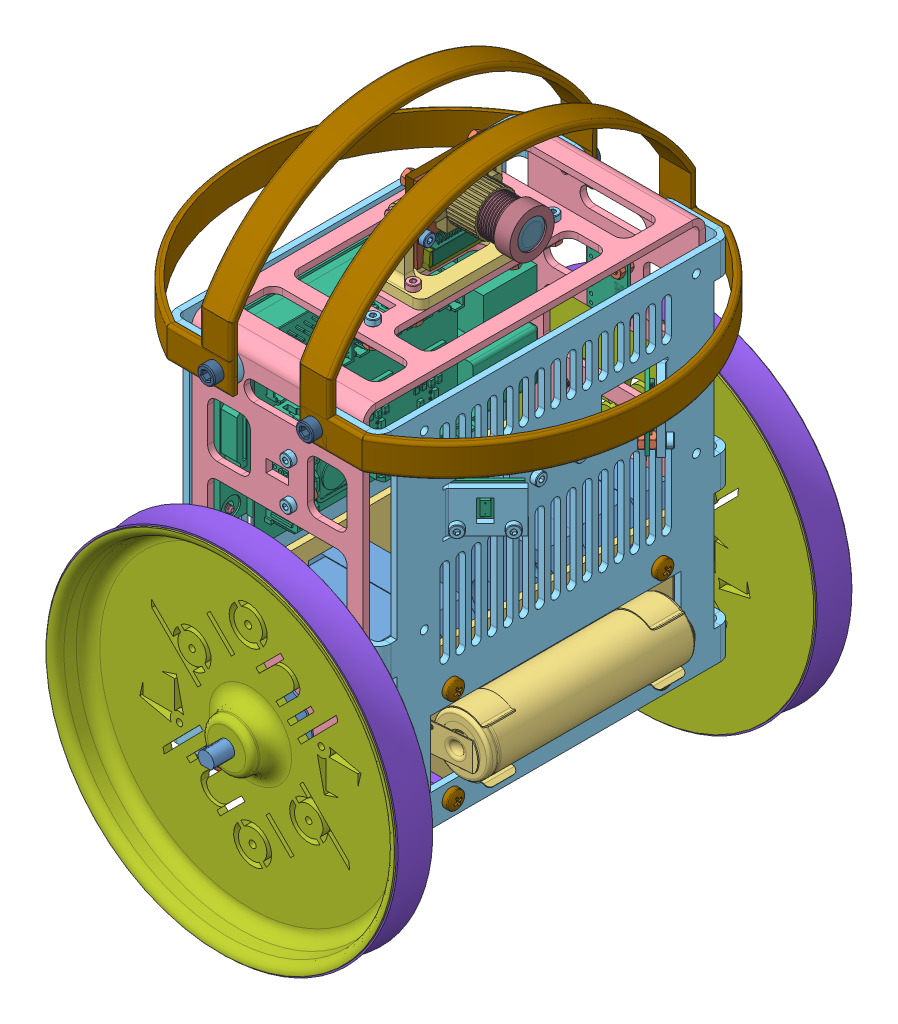
SolidWorks assembly irys4, configuration Domyślna. Lengths in mm. (continued)
Mates (geometry in assembly coordinates): (continued)
- Koncentryczne66: concentric aligned: cylinder of bumper-2 through (-57.7578 82.3211 -37.682) axis (0 0 1) radius 1.5; cylinder of bumper-4 through (-57.7578 82.3211 -37.75) axis (0 0 1) radius 1.5
- Wspólnie32: coincident: line of front-1 through (-57.7578 77.3211 -35.75) axis (-1 0 0); plane of bumper-4 through (-52.7604 77.3184 -35.75) normal (0 0 1)
- Koncentryczne67: concentric aligned: cylinder of bumper-3 through (-26.7578 82.3211 -37.75) axis (0 0 1) radius 1.5; cylinder of bumper-5 through (-26.7578 82.3211 -37.75) axis (0 0 1) radius 1.5
- Wspólnie33: coincident: line of front-2 through (-26.7578 87.3211 -35.75) axis (1 0 0); plane of bumper-5 through (-21.7734 77.3055 -35.75) normal (0 0 1)
- Wspólnie34: coincident anti-aligned: plane of topframe-1 through (-42.2578 90.6087 -127.75) normal (0 1 0); plane of camera_mounted-1/mount1-1 through (-40.7578 90.6087 2.1027) normal (0 -1 0)
- Koncentryczne70: concentric aligned: cylinder of front-2 through (0.677 52.3211 42.6028) axis (0.707107 0 0.707107) radius 1.25; cylinder of m2_x_0_4mm_thread_6mm_long_sock-2 through (3.5055 52.3211 45.4313) axis (0.707107 0 0.707107) radius 1.9
- Wspólnie35: coincident anti-aligned: plane of front-2 through (-34.9258 82.3211 81.0341) normal (0.707107 0 0.707107); plane of m2_x_0_4mm_thread_6mm_long_sock-2 through (2.0912 52.3211 44.017) normal (-0.707107 0 -0.707107)
- Koncentryczne71: concentric aligned: cylinder of front-2 through (-8.3032 52.3211 51.5831) axis (0.707107 0 0.707107) radius 1.25; cylinder of m2_x_0_4mm_thread_6mm_long_sock-1 through (-5.4748 52.3211 54.4115) axis (0.707107 0 0.707107) radius 1.9
- Wspólnie36: coincident anti-aligned: plane of front-2 through (-34.9258 82.3211 81.0341) normal (0.707107 0 0.707107); plane of m2_x_0_4mm_thread_6mm_long_sock-1 through (-6.889 52.3211 52.9973) normal (-0.707107 0 -0.707107)
- Koncentryczne76: concentric aligned: cylinder of front-1 through (-77.0454 33.0917 64.6663) axis (1 0 0) radius 1.25; cylinder of M2 x 0.4mm Thread 10mm LONG SOCKET HEAD CAP SCREW-1 through (-78.0454 33.0917 64.6663) axis (1 0 0) radius 1.9
- Wspólnie43: coincident anti-aligned: plane of front-1 through (-76.0454 82.3211 -50.75) normal (-1 0 0); plane of M2 x 0.4mm Thread 10mm LONG SOCKET HEAD CAP SCREW-1 through (-76.0454 33.0917 64.6663) normal (1 0 0)
- Koncentryczne77: concentric aligned: cylinder of front-1 through (-77.0454 82.1645 64.6663) axis (1 0 0) radius 1.25; cylinder of M2 x 0.4mm Thread 10mm LONG SOCKET HEAD CAP SCREW-2 through (-78.0454 82.1645 64.6663) axis (1 0 0) radius 1.9
- Wspólnie44: coincident anti-aligned: plane of front-1 through (-76.0454 82.3211 -50.75) normal (-1 0 0); plane of M2 x 0.4mm Thread 10mm LONG SOCKET HEAD CAP SCREW-2 through (-76.0454 82.1645 64.6663) normal (1 0 0)
- Koncentryczne82: concentric anti-aligned: cylinder of m2_x_0_4mm_thread_6mm_long_sock-2 through (3.5055 52.3211 45.4313) axis (0.707107 0 0.707107) radius 1.9; cylinder of ToF_nut-1/m2_x_0_4mm_thread_hex_nut-1 through (-2.307 52.3211 39.6188) axis (-0.707107 0 -0.707107) radius 0.7402
- Koncentryczne83: concentric anti-aligned: cylinder of m2_x_0_4mm_thread_6mm_long_sock-1 through (-5.4748 52.3211 54.4115) axis (0.707107 0 0.707107) radius 1.9; cylinder of ToF_nut-1/m2_x_0_4mm_thread_hex_nut-4 through (-9.4346 52.3211 50.4517) axis (-0.707107 0 -0.707107) radius 1
- Wspólnie49: coincident anti-aligned: plane of front-2 through (-36.34 82.3211 79.6199) normal (-0.707107 0 -0.707107); plane of ToF_nut-1/m2_x_0_4mm_thread_hex_nut-3 through (1.973 50.9159 41.3069) normal (0.707107 0 0.707107)
- Koncentryczne84: concentric aligned: cylinder of front-2 through (0.9091 52.3211 -2.1989) axis (0.707107 0 -0.707107) radius 1.25; cylinder of ToF_nut-2/m2_x_0_4mm_thread_hex_nut-2 through (-0.9436 52.3211 -0.3463) axis (0.707107 0 -0.707107) radius 0.7402
- Koncentryczne85: concentric aligned: cylinder of front-2 through (-8.0712 52.3211 -11.1792) axis (0.707107 0 -0.707107) radius 1.25; cylinder of ToF_nut-2/m2_x_0_4mm_thread_hex_nut-3 through (-8.0712 52.3211 -11.1792) axis (0.707107 0 -0.707107) radius 0.7402
- Wspólnie51: coincident anti-aligned: plane of front-2 through (64.3012 82.3211 61.1932) normal (-0.707107 0 0.707107); plane of ToF_nut-2/m2_x_0_4mm_thread_hex_nut-4 through (-0.3869 50.9159 -3.4949) normal (0.707107 0 -0.707107)
- Koncentryczne86: concentric aligned: cylinder of front-2 through (-10.4701 52.3211 26.6) axis (1 0 0) radius 1.25; cylinder of ToF_nut-3/m2_x_0_4mm_thread_hex_nut-4 through (-10.4701 52.3211 26.6) axis (1 0 0) radius 0.7402
- Koncentryczne87: concentric aligned: cylinder of front-2 through (-10.4701 52.3211 13.9) axis (1 0 0) radius 1.25; cylinder of ToF_nut-3/m2_x_0_4mm_thread_hex_nut-3 through (-10.4701 52.3211 13.9) axis (1 0 0) radius 0.7402
- Wspólnie52: coincident anti-aligned: plane of front-2 through (-10.4701 82.3211 91.25) normal (-1 0 0); plane of ToF_nut-3/m2_x_0_4mm_thread_hex_nut-3 through (-10.4701 50.9159 12.0673) normal (1 0 0)
- Koncentryczne92: concentric aligned: cylinder of front-2 through (-8.0712 52.3211 -11.1792) axis (0.707107 0 -0.707107) radius 1.25; cylinder of m2_x_0_4mm_thread_6mm_long_sock-4 through (-5.2428 52.3211 -14.0076) axis (0.707107 0 -0.707107) radius 1.9
- Koncentryczne93: concentric aligned: cylinder of front-2 through (0.9091 52.3211 -2.1989) axis (0.707107 0 -0.707107) radius 1.25; cylinder of m2_x_0_4mm_thread_6mm_long_sock-6 through (3.7375 52.3211 -5.0274) axis (0.707107 0 -0.707107) radius 1.9
- Koncentryczne94: concentric aligned: cylinder of front-2 through (-10.4701 52.3211 13.9) axis (1 0 0) radius 1.25; cylinder of m2_x_0_4mm_thread_6mm_long_sock-3 through (-6.4701 52.3211 13.9) axis (1 0 0) radius 1.9
- Koncentryczne95: concentric aligned: cylinder of front-2 through (-10.4701 52.3211 26.6) axis (1 0 0) radius 1.25; cylinder of m2_x_0_4mm_thread_6mm_long_sock-5 through (-6.4701 52.3211 26.6) axis (1 0 0) radius 1.9
- Wspólnie55: coincident anti-aligned: plane of front-2 through (-8.4701 82.3211 91.25) normal (1 0 0); plane of m2_x_0_4mm_thread_6mm_long_sock-5 through (-8.4701 52.3211 26.6) normal (-1 0 0)
- Wspólnie57: coincident anti-aligned: plane of front-2 through (65.7154 82.3211 59.779) normal (0.707107 0 -0.707107); plane of m2_x_0_4mm_thread_6mm_long_sock-4 through (-6.657 52.3211 -12.5934) normal (-0.707107 0 0.707107)
- Wspólnie58: coincident: plane of front-2 through (65.7154 82.3211 59.779) normal (0.707107 0 -0.707107); moEndPointRef_w of m2_x_0_4mm_thread_6mm_long_sock-6
- Wspólnie59: coincident anti-aligned: plane of front-2 through (-8.4701 82.3211 91.25) normal (1 0 0); plane of m2_x_0_4mm_thread_6mm_long_sock-3 through (-8.4701 52.3211 13.9) normal (-1 0 0)
- Koncentryczne96: concentric aligned: cylinder of topframe-1 through (-37.7578 90.6087 -8.1) axis (0 1 0) radius 1.25; cylinder of ToF_nut-4/m2_x_0_4mm_thread_hex_nut-3 through (-37.7578 88.6087 -8.1) axis (0 1 0) radius 0.7402
- Koncentryczne97: concentric aligned: cylinder of camera_mounted-1/mount1-1 through (-37.7578 90.6087 4.6) axis (0 1 0) radius 1.05; cylinder of ToF_nut-4/m2_x_0_4mm_thread_hex_nut-4 through (-37.7578 88.6087 4.6) axis (0 1 0) radius 0.7402
- Wspólnie60: coincident anti-aligned: plane of topframe-1 through (-42.2578 88.6087 -127.75) normal (0 -1 0); plane of ToF_nut-4/m2_x_0_4mm_thread_hex_nut-3 through (-36.3526 88.6087 -9.9327) normal (0 1 0)
- Koncentryczne98: concentric aligned: cylinder of topframe-1 through (-37.7578 90.6087 48.6) axis (0 1 0) radius 1.25; cylinder of ToF_nut-5/m2_x_0_4mm_thread_hex_nut-4 through (-37.7578 88.6087 48.6) axis (0 1 0) radius 0.7402
- Koncentryczne99: concentric aligned: cylinder of camera_mounted-1/mount1-1 through (-37.7578 90.6087 35.9) axis (0 1 0) radius 1.05; cylinder of ToF_nut-5/m2_x_0_4mm_thread_hex_nut-3 through (-37.7578 88.6087 35.9) axis (0 1 0) radius 0.7402
- Wspólnie61: coincident anti-aligned: plane of topframe-1 through (-42.2578 88.6087 -127.75) normal (0 -1 0); plane of ToF_nut-5/m2_x_0_4mm_thread_hex_nut-4 through (-36.3526 88.6087 46.7673) normal (0 1 0)
- Koncentryczne100: concentric anti-aligned: cylinder of camera_mounted-1/mount1-1 through (-37.7578 90.6087 35.9) axis (0 1 0) radius 1.05; cylinder of M2 x 0.4mm Thread 10mm LONG SOCKET HEAD CAP SCREW-4 through (-37.7578 95.6087 35.9) axis (0 -1 0) radius 1.9
- Koncentryczne102: concentric anti-aligned: cylinder of camera_mounted-1/mount1-1 through (-37.7578 90.6087 4.6) axis (0 1 0) radius 1.05; cylinder of M2 x 0.4mm Thread 10mm LONG SOCKET HEAD CAP SCREW-3 through (-37.7578 95.6087 4.6) axis (0 -1 0) radius 1.9
- Wspólnie62: coincident anti-aligned: plane of camera_mounted-1/mount1-1 through (-40.7578 93.6087 7.7527) normal (0 1 0); plane of M2 x 0.4mm Thread 10mm LONG SOCKET HEAD CAP SCREW-3 through (-37.7578 93.6087 4.6) normal (0 -1 0)
- Wspólnie64: coincident anti-aligned: plane of camera_mounted-1/mount1-1 through (-40.7578 93.6087 7.7527) normal (0 1 0); plane of M2 x 0.4mm Thread 10mm LONG SOCKET HEAD CAP SCREW-4 through (-37.7578 93.6087 35.9) normal (0 -1 0)
- Koncentryczne103: concentric aligned: cylinder of topframe-1 through (-37.7578 90.6087 -8.1) axis (0 1 0) radius 1.25; cylinder of m2_x_0_4mm_thread_6mm_long_sock-8 through (-37.7578 92.6087 -8.1) axis (0 1 0) radius 1.9
- Koncentryczne104: concentric aligned: cylinder of topframe-1 through (-37.7578 90.6087 48.6) axis (0 1 0) radius 1.25; cylinder of m2_x_0_4mm_thread_6mm_long_sock-7 through (-37.7578 92.6087 48.6) axis (0 1 0) radius 1.9
- Wspólnie65: coincident anti-aligned: plane of topframe-1 through (-42.2578 90.6087 -127.75) normal (0 1 0); plane of m2_x_0_4mm_thread_6mm_long_sock-7 through (-37.7578 90.6087 48.6) normal (0 -1 0)
- Wspólnie66: coincident anti-aligned: plane of topframe-1 through (-42.2578 90.6087 -127.75) normal (0 1 0); plane of m2_x_0_4mm_thread_6mm_long_sock-8 through (-37.7578 90.6087 -8.1) normal (0 -1 0)
- Koncentryczne105: concentric anti-aligned: cylinder of topframe-1 through (-37.7578 66.6711 74.25) axis (0 0 1) radius 1.25; cylinder of ToF_nut-6/m2_x_0_4mm_thread_hex_nut-3 through (-37.7578 66.6711 70.65) axis (0 0 -1) radius 1
- Koncentryczne106: concentric aligned: cylinder of topframe-1 through (-37.7578 53.9711 74.25) axis (0 0 1) radius 1.25; cylinder of ToF_nut-6/m2_x_0_4mm_thread_hex_nut-4 through (-37.7578 53.9711 72.25) axis (0 0 1) radius 0.7402
- Wspólnie67: coincident anti-aligned: plane of topframe-1 through (-42.2578 289.3211 72.25) normal (0 0 -1); plane of ToF_nut-6/m2_x_0_4mm_thread_hex_nut-4 through (-36.3526 55.8038 72.25) normal (0 0 1)
- Koncentryczne107: concentric anti-aligned: cylinder of topframe-1 through (-37.7578 53.9711 -33.75) axis (0 0 -1) radius 1.25; cylinder of ToF_nut-7/vl53l1x-1 through (-37.7578 53.9711 -30.15) axis (0 0 1) radius 1.0922
- Koncentryczne108: concentric aligned: cylinder of topframe-1 through (-37.7578 66.6711 -33.75) axis (0 0 -1) radius 1.25; cylinder of ToF_nut-7/m2_x_0_4mm_thread_hex_nut-4 through (-37.7578 66.6711 -31.75) axis (0 0 -1) radius 0.7402
- Wspólnie68: coincident anti-aligned: plane of topframe-1 through (-42.2578 -6.6789 -31.75) normal (0 0 1); plane of ToF_nut-7/m2_x_0_4mm_thread_hex_nut-3 through (-36.3526 52.1384 -31.75) normal (0 0 -1)
- Koncentryczne109: concentric aligned: cylinder of front-1 through (-76.2123 52.3211 -11.0831) axis (-0.707107 0 -0.707107) radius 1.25; cylinder of ToF_nut-8/m2_x_0_4mm_thread_hex_nut-4 through (-76.2123 52.3211 -11.0831) axis (-0.707107 0 -0.707107) radius 0.7402
- Koncentryczne110: concentric anti-aligned: cylinder of front-1 through (-85.1925 52.3211 -2.1028) axis (-0.707107 0 -0.707107) radius 1.25; cylinder of ToF_nut-8/m2_x_0_4mm_thread_hex_nut-3 through (-84.0612 52.3211 -0.9715) axis (0.707107 0 0.707107) radius 1
- Wspólnie69: coincident anti-aligned: plane of front-1 through (-48.1755 82.3211 -39.1199) normal (0.707107 0 0.707107); plane of ToF_nut-8/m2_x_0_4mm_thread_hex_nut-3 through (-86.4885 50.9159 -0.8069) normal (-0.707107 0 -0.707107)
- Koncentryczne111: concentric aligned: cylinder of front-1 through (-74.0454 52.3211 13.9) axis (-1 0 0) radius 1.25; cylinder of ToF_nut-9/m2_x_0_4mm_thread_hex_nut-4 through (-74.0454 52.3211 13.9) axis (-1 0 0) radius 0.7402
- Koncentryczne112: concentric aligned: cylinder of front-1 through (-74.0454 52.3211 26.6) axis (-1 0 0) radius 1.25; cylinder of ToF_nut-9/m2_x_0_4mm_thread_hex_nut-3 through (-74.0454 52.3211 26.6) axis (-1 0 0) radius 0.7402
- Wspólnie70: coincident anti-aligned: plane of front-1 through (-74.0454 82.3211 -50.75) normal (1 0 0); plane of ToF_nut-9/m2_x_0_4mm_thread_hex_nut-4 through (-74.0454 50.9159 15.7327) normal (-1 0 0)
- Koncentryczne113: concentric aligned: cylinder of front-1 through (-76.4443 52.3211 51.6792) axis (-0.707107 0 0.707107) radius 1.25; cylinder of ToF_nut-10/m2_x_0_4mm_thread_hex_nut-3 through (-76.4443 52.3211 51.6792) axis (-0.707107 0 0.707107) radius 0.7402
- Koncentryczne114: concentric aligned: cylinder of front-1 through (-85.4246 52.3211 42.6989) axis (-0.707107 0 0.707107) radius 1.25; cylinder of ToF_nut-10/m2_x_0_4mm_thread_hex_nut-4 through (-85.4246 52.3211 42.6989) axis (-0.707107 0 0.707107) radius 0.7402
- Wspólnie71: coincident anti-aligned: plane of front-1 through (-148.8167 82.3211 -20.6932) normal (0.707107 0 -0.707107); plane of ToF_nut-10/m2_x_0_4mm_thread_hex_nut-4 through (-84.1286 50.9159 43.9949) normal (-0.707107 0 0.707107)
- Koncentryczne115: concentric aligned: cylinder of front-1 through (-76.2123 52.3211 -11.0831) axis (-0.707107 0 -0.707107) radius 1.25; cylinder of m2_x_0_4mm_thread_6mm_long_sock-9 through (-79.0407 52.3211 -13.9115) axis (-0.707107 0 -0.707107) radius 1.9
- Koncentryczne116: concentric aligned: cylinder of front-1 through (-85.1925 52.3211 -2.1028) axis (-0.707107 0 -0.707107) radius 1.25; cylinder of m2_x_0_4mm_thread_6mm_long_sock-10 through (-88.021 52.3211 -4.9313) axis (-0.707107 0 -0.707107) radius 1.9
- Wspólnie72: coincident anti-aligned: plane of front-1 through (-49.5897 82.3211 -40.5341) normal (-0.707107 0 -0.707107); plane of m2_x_0_4mm_thread_6mm_long_sock-9 through (-77.6265 52.3211 -12.4973) normal (0.707107 0 0.707107)
- Wspólnie73: coincident anti-aligned: plane of front-1 through (-49.5897 82.3211 -40.5341) normal (-0.707107 0 -0.707107); plane of m2_x_0_4mm_thread_6mm_long_sock-10 through (-86.6068 52.3211 -3.517) normal (0.707107 0 0.707107)
- Koncentryczne117: concentric aligned: cylinder of front-1 through (-74.0454 52.3211 13.9) axis (-1 0 0) radius 1.25; cylinder of m2_x_0_4mm_thread_6mm_long_sock-11 through (-78.0454 52.3211 13.9) axis (-1 0 0) radius 1.9
- Koncentryczne118: concentric aligned: cylinder of front-1 through (-74.0454 52.3211 26.6) axis (-1 0 0) radius 1.25; cylinder of m2_x_0_4mm_thread_6mm_long_sock-12 through (-78.0454 52.3211 26.6) axis (-1 0 0) radius 1.9
- Wspólnie74: coincident anti-aligned: plane of front-1 through (-76.0454 82.3211 -50.75) normal (-1 0 0); plane of m2_x_0_4mm_thread_6mm_long_sock-11 through (-76.0454 52.3211 13.9) normal (1 0 0)
- Wspólnie75: coincident anti-aligned: plane of front-1 through (-76.0454 82.3211 -50.75) normal (-1 0 0); plane of m2_x_0_4mm_thread_6mm_long_sock-12 through (-76.0454 52.3211 26.6) normal (1 0 0)
- Koncentryczne119: concentric aligned: cylinder of front-1 through (-85.4246 52.3211 42.6989) axis (-0.707107 0 0.707107) radius 1.25; cylinder of m2_x_0_4mm_thread_6mm_long_sock-13 through (-88.253 52.3211 45.5274) axis (-0.707107 0 0.707107) radius 1.9
- Koncentryczne120: concentric aligned: cylinder of front-1 through (-76.4443 52.3211 51.6792) axis (-0.707107 0 0.707107) radius 1.25; cylinder of m2_x_0_4mm_thread_6mm_long_sock-14 through (-79.2728 52.3211 54.5076) axis (-0.707107 0 0.707107) radius 1.9
- Wspólnie76: coincident anti-aligned: plane of front-1 through (-150.2309 82.3211 -19.279) normal (-0.707107 0 0.707107); plane of m2_x_0_4mm_thread_6mm_long_sock-13 through (-86.8388 52.3211 44.1132) normal (0.707107 0 -0.707107)
- Wspólnie77: coincident anti-aligned: plane of front-1 through (-150.2309 82.3211 -19.279) normal (-0.707107 0 0.707107); plane of m2_x_0_4mm_thread_6mm_long_sock-14 through (-77.8585 52.3211 53.0934) normal (0.707107 0 -0.707107)
- Koncentryczne121: concentric aligned: cylinder of topframe-1 through (-37.7578 53.9711 74.25) axis (0 0 1) radius 1.25; cylinder of m2_x_0_4mm_thread_6mm_long_sock-16 through (-37.7578 53.9711 76.25) axis (0 0 1) radius 1.9
- Koncentryczne122: concentric aligned: cylinder of topframe-1 through (-37.7578 66.6711 74.25) axis (0 0 1) radius 1.25; cylinder of m2_x_0_4mm_thread_6mm_long_sock-15 through (-37.7578 66.6711 76.25) axis (0 0 1) radius 1.9
- Wspólnie78: coincident anti-aligned: plane of topframe-1 through (-42.2578 289.3211 74.25) normal (0 0 1); plane of m2_x_0_4mm_thread_6mm_long_sock-15 through (-37.7578 66.6711 74.25) normal (0 0 -1)
- Wspólnie79: coincident anti-aligned: plane of topframe-1 through (-42.2578 289.3211 74.25) normal (0 0 1); plane of m2_x_0_4mm_thread_6mm_long_sock-16 through (-37.7578 53.9711 74.25) normal (0 0 -1)
- Koncentryczne123: concentric aligned: cylinder of topframe-1 through (-37.7578 53.9711 -33.75) axis (0 0 -1) radius 1.25; cylinder of m2_x_0_4mm_thread_6mm_long_sock-18 through (-37.7578 53.9711 -35.75) axis (0 0 -1) radius 1.9
- Koncentryczne124: concentric aligned: cylinder of topframe-1 through (-37.7578 66.6711 -33.75) axis (0 0 -1) radius 1.25; cylinder of m2_x_0_4mm_thread_6mm_long_sock-17 through (-37.7578 66.6711 -35.75) axis (0 0 -1) radius 1.9
- Wspólnie80: coincident anti-aligned: plane of topframe-1 through (-42.2578 -6.6789 -33.75) normal (0 0 -1); plane of m2_x_0_4mm_thread_6mm_long_sock-17 through (-37.7578 66.6711 -33.75) normal (0 0 1)
- Wspólnie81: coincident anti-aligned: plane of topframe-1 through (-42.2578 -6.6789 -33.75) normal (0 0 -1); plane of m2_x_0_4mm_thread_6mm_long_sock-18 through (-37.7578 53.9711 -33.75) normal (0 0 1)
- Koncentryczne125: concentric aligned: cylinder of battery_module-1 through (-51.2078 -28.4959 17.65) axis (0 1 0) radius 1.1; cylinder of H-H_M3x12mm-1 through (-51.2078 -28.4959 17.65) axis (0 1 0) radius 1.5
- Wspólnie82: coincident anti-aligned: plane of battery_module-1 through (-62.2578 -28.4959 65.25) normal (0 1 0); plane of H-H_M3x12mm-1 through (-51.2078 -28.4959 17.65) normal (0 -1 0)
- Wspólnie83: coincident anti-aligned: circle of H-H_M3x12mm-1; cylinder of H-H_M3x6mm-1 through (-51.2078 -16.4959 17.65) axis (0 1 0) radius 1.5
- Wspólnie84: coincident anti-aligned: plane of H-H_M3x12mm-1 through (-51.2078 -16.4959 17.65) normal (0 1 0); plane of H-H_M3x6mm-1 through (-51.2078 -16.4959 17.65) normal (0 -1 0)
- Wspólnie85: coincident anti-aligned: plane of imu-1 through (-53.5985 -10.4959 25.3181) normal (0 -1 0); plane of H-H_M3x6mm-1 through (-51.2078 -10.4959 17.65) normal (0 1 0)
- Koncentryczne1261: concentric aligned: cylinder of imu-1 through (-51.2078 -10.4959 17.65) axis (0 1 0) radius 1.0922; cylinder of pan cross head_am-2 through (-51.2078 18.3201 17.65) axis (0 1 0) radius 2.8
- Wspólnie871: coincident anti-aligned: plane of imu-1 through (-53.5985 -9.4799 25.3181) normal (0 1 0); plane of pan cross head_am-2 through (-49.7078 -9.4799 17.65) normal (0 -1 0)
- Koncentryczne127: concentric aligned: cylinder of front-1 through (-74.0454 7.8211 -12.75) axis (-1 0 0) radius 1.4; cylinder of battery_module_H-2/H-H_M3x6mm-1 through (-68.0454 7.8211 -12.75) axis (-1 0 0) radius 1.5
- Koncentryczne128: concentric aligned: cylinder of front-1 through (-74.0454 -22.1789 53.25) axis (-1 0 0) radius 1.4; cylinder of battery_module_H-2/H-H_M3x6mm-4 through (-68.0454 -22.1789 53.25) axis (-1 0 0) radius 1.5
- Wspólnie88: coincident anti-aligned: plane of front-1 through (-74.0454 82.3211 -50.75) normal (1 0 0); plane of battery_module_H-2/H-H_M3x6mm-1 through (-74.0454 7.8211 -12.75) normal (-1 0 0)
- Koncentryczne1291: concentric aligned: cylinder of front-1 through (-74.0454 -22.1789 53.25) axis (-1 0 0) radius 1.4; cylinder of pan cross head_am-3 through (-103.8454 -22.1789 53.25) axis (-1 0 0) radius 2.8
- Wspólnie891: coincident anti-aligned: plane of front-1 through (-76.0454 82.3211 -50.75) normal (-1 0 0); plane of pan cross head_am-3 through (-76.0454 -20.6789 53.25) normal (1 0 0)
- Koncentryczne1301: concentric aligned: cylinder of front-1 through (-74.0454 7.8211 53.25) axis (-1 0 0) radius 1.4; cylinder of pan cross head_am-4 through (-103.8454 7.8211 53.25) axis (-1 0 0) radius 2.8
- Wspólnie901: coincident anti-aligned: plane of front-1 through (-76.0454 82.3211 -50.75) normal (-1 0 0); plane of pan cross head_am-4 through (-76.0454 9.3211 53.25) normal (1 0 0)
- Koncentryczne1311: concentric aligned: cylinder of front-1 through (-74.0454 7.8211 -12.75) axis (-1 0 0) radius 1.4; cylinder of pan cross head_am-5 through (-103.8454 7.8211 -12.75) axis (-1 0 0) radius 2.8
- Wspólnie911: coincident anti-aligned: plane of front-1 through (-76.0454 82.3211 -50.75) normal (-1 0 0); plane of pan cross head_am-5 through (-76.0454 9.3211 -12.75) normal (1 0 0)
- Koncentryczne1321: concentric aligned: cylinder of front-1 through (-74.0454 -22.1789 -12.75) axis (-1 0 0) radius 1.4; cylinder of pan cross head_am-6 through (-103.8454 -22.1789 -12.75) axis (-1 0 0) radius 2.8
- Wspólnie921: coincident anti-aligned: plane of front-1 through (-76.0454 82.3211 -50.75) normal (-1 0 0); plane of pan cross head_am-6 through (-76.0454 -20.6789 -12.75) normal (1 0 0)
- Koncentryczne1331: concentric aligned: cylinder of bottomframe_rys3-1 through (-57.2578 -32.5373 53.25) axis (0 -1 0) radius 1.4; cylinder of pan cross head_am-7 through (-57.2578 -60.3373 53.25) axis (0 -1 0) radius 2.8
- Wspólnie931: coincident anti-aligned: plane of bottomframe_rys3-1 through (-42.2578 -32.5373 96.25) normal (0 -1 0); plane of pan cross head_am-7 through (-58.7578 -32.5373 53.25) normal (0 1 0)
- Koncentryczne1341: concentric aligned: cylinder of bottomframe_rys3-1 through (-27.2578 -32.5373 53.25) axis (0 -1 0) radius 1.4; cylinder of pan cross head_am-8 through (-27.2578 -60.3373 53.25) axis (0 -1 0) radius 2.8
- Wspólnie941: coincident anti-aligned: plane of bottomframe_rys3-1 through (-42.2578 -32.5373 96.25) normal (0 -1 0); plane of pan cross head_am-8 through (-28.7578 -32.5373 53.25) normal (0 1 0)
- Koncentryczne1351: concentric aligned: cylinder of bottomframe_rys3-1 through (-57.2578 -32.5373 -12.75) axis (0 -1 0) radius 1.4; cylinder of pan cross head_am-9 through (-57.2578 -60.3373 -12.75) axis (0 -1 0) radius 2.8
- Wspólnie951: coincident anti-aligned: plane of bottomframe_rys3-1 through (-42.2578 -32.5373 96.25) normal (0 -1 0); plane of pan cross head_am-9 through (-58.7578 -32.5373 -12.75) normal (0 1 0)
- Koncentryczne1361: concentric aligned: cylinder of bottomframe_rys3-1 through (-27.2578 -32.5373 -12.75) axis (0 -1 0) radius 1.4; cylinder of pan cross head_am-10 through (-27.2578 -60.3373 -12.75) axis (0 -1 0) radius 2.8
- Wspólnie961: coincident anti-aligned: plane of bottomframe_rys3-1 through (-42.2578 -32.5373 96.25) normal (0 -1 0); plane of pan cross head_am-10 through (-28.7578 -32.5373 -12.75) normal (0 1 0)
- Koncentryczne138: concentric aligned: cylinder of front-2 through (-10.4701 -22.1789 -12.75) axis (1 0 0) radius 1.4; cylinder of battery_module_H-3/H-H_M3x6mm-1 through (-16.4701 -22.1789 -12.75) axis (1 0 0) radius 1.5
- Koncentryczne139: concentric aligned: cylinder of front-2 through (-10.4701 7.8211 53.25) axis (1 0 0) radius 1.4; cylinder of battery_module_H-3/H-H_M3x6mm-4 through (-16.4701 7.8211 53.25) axis (1 0 0) radius 1.5
- Wspólnie98: coincident anti-aligned: plane of front-2 through (-10.4701 82.3211 91.25) normal (-1 0 0); plane of battery_module_H-3/H-H_M3x6mm-3 through (-10.4701 7.8211 -12.75) normal (1 0 0)
- Koncentryczne1401: concentric aligned: cylinder of front-2 through (-10.4701 -22.1789 53.25) axis (1 0 0) radius 1.4; cylinder of pan cross head_am-11 through (19.3299 -22.1789 53.25) axis (1 0 0) radius 2.8
- Wspólnie991: coincident anti-aligned: plane of front-2 through (-8.4701 82.3211 91.25) normal (1 0 0); plane of pan cross head_am-11 through (-8.4701 -22.7517 54.6363) normal (-1 0 0)
- Koncentryczne1411: concentric aligned: cylinder of front-2 through (-10.4701 7.8211 53.25) axis (1 0 0) radius 1.4; cylinder of pan cross head_am-12 through (19.3299 7.8211 53.25) axis (1 0 0) radius 2.8
- Wspólnie1001: coincident anti-aligned: plane of front-2 through (-8.4701 82.3211 91.25) normal (1 0 0); plane of pan cross head_am-12 through (-8.4701 7.2483 54.6363) normal (-1 0 0)
- Koncentryczne1421: concentric aligned: cylinder of front-2 through (-10.4701 7.8211 -12.75) axis (1 0 0) radius 1.4; cylinder of pan cross head_am-13 through (19.3299 7.8211 -12.75) axis (1 0 0) radius 2.8
- Wspólnie1011: coincident anti-aligned: plane of front-2 through (-8.4701 82.3211 91.25) normal (1 0 0); plane of pan cross head_am-13 through (-8.4701 7.2483 -11.3637) normal (-1 0 0)
- Koncentryczne1431: concentric aligned: cylinder of front-2 through (-10.4701 -22.1789 -12.75) axis (1 0 0) radius 1.4; cylinder of pan cross head_am-14 through (19.3299 -22.1789 -12.75) axis (1 0 0) radius 2.8
- Wspólnie1021: coincident anti-aligned: plane of front-2 through (-8.4701 82.3211 91.25) normal (1 0 0); plane of pan cross head_am-14 through (-8.4701 -22.7517 -11.3637) normal (-1 0 0)
- Koncentryczne144: concentric aligned: cylinder of front-1 through (-57.7578 82.3211 -33.75) axis (0 0 -1) radius 1.75; cylinder of M3x6-1 through (-57.7578 82.3211 -129.4555) axis (0 0 -1) radius 2.75
- Wspólnie103: coincident anti-aligned: plane of bumper-4 through (-52.7604 77.3184 -37.75) normal (0 0 -1); plane of M3x6-1 through (-57.187 80.9447 -37.75) normal (0 0 1)
- Koncentryczne145: concentric aligned: cylinder of front-2 through (-26.7578 82.3211 -33.75) axis (0 0 -1) radius 1.75; cylinder of M3x6-2 through (-26.7578 82.3211 -129.4555) axis (0 0 -1) radius 2.75
- Wspólnie104: coincident anti-aligned: plane of bumper-3 through (-31.7578 77.3211 -37.75) normal (0 0 -1); plane of M3x6-2 through (-26.187 80.9447 -37.75) normal (0 0 1)
- Koncentryczne146: concentric aligned: cylinder of front-2 through (-26.7578 24.3211 -33.75) axis (0 0 -1) radius 1.75; cylinder of M3x4-1 through (-26.7578 24.3211 -127.4555) axis (0 0 -1) radius 2.75
- Koncentryczne147: concentric aligned: cylinder of front-1 through (-57.7578 24.3211 -33.75) axis (0 0 -1) radius 1.75; cylinder of M3x4-2 through (-57.7578 24.3211 -127.4555) axis (0 0 -1) radius 2.75
- Wspólnie105: coincident anti-aligned: plane of front-1 through (-57.7578 82.3211 -35.75) normal (0 0 -1); plane of M3x4-2 through (-57.187 22.9447 -35.75) normal (0 0 1)
- Wspólnie106: coincident anti-aligned: plane of front-2 through (115.2422 82.3211 -35.75) normal (0 0 -1); plane of M3x4-1 through (-26.187 22.9447 -35.75) normal (0 0 1)
- Koncentryczne148: concentric aligned: cylinder of topframe-1 through (-26.7578 8.3211 -33.75) axis (0 0 -1) radius 1.6; cylinder of M3x8-1 through (-26.7578 8.3211 -125.4555) axis (0 0 -1) radius 2.75
- Wspólnie107: coincident anti-aligned: plane of topframe-1 through (-42.2578 -6.6789 -33.75) normal (0 0 -1); plane of M3x8-1 through (-26.187 6.9447 -33.75) normal (0 0 1)
- Koncentryczne149: concentric aligned: cylinder of topframe-1 through (-57.7578 8.3211 -33.75) axis (0 0 -1) radius 1.6; cylinder of M3x8-2 through (-57.7578 8.3211 -125.4555) axis (0 0 -1) radius 2.75
- Wspólnie108: coincident anti-aligned: plane of topframe-1 through (-42.2578 -6.6789 -33.75) normal (0 0 -1); plane of M3x8-2 through (-57.187 6.9447 -33.75) normal (0 0 1)
- Koncentryczne150: concentric aligned: cylinder of bottomframe_rys3-1 through (-57.7578 -22.6789 -33.75) axis (0 0 -1) radius 1.6; cylinder of M3x8-4 through (-57.7578 -22.6789 -127.4555) axis (0 0 -1) radius 2.75
- Koncentryczne151: concentric aligned: cylinder of front-2 through (-26.7578 -22.6789 -33.75) axis (0 0 -1) radius 1.75; cylinder of M3x8-3 through (-26.7578 -22.6789 -127.4555) axis (0 0 -1) radius 2.75
- Wspólnie109: coincident anti-aligned: plane of front-1 through (-57.7578 82.3211 -35.75) normal (0 0 -1); plane of M3x8-4 through (-57.187 -24.0553 -35.75) normal (0 0 1)
- Wspólnie110: coincident aligned: plane of front-2 through (115.2422 82.3211 -35.75) normal (0 0 -1); circle of M3x8-3
- Koncentryczne152: concentric aligned: cylinder of front-2 through (-26.7578 82.3211 74.25) axis (0 0 1) radius 1.75; cylinder of M3x6-4 through (-26.7578 82.3211 169.9555) axis (0 0 1) radius 2.75
- Koncentryczne153: concentric aligned: circle of topframe-1; cylinder of M3x6-3 through (-57.7578 82.3211 170.0235) axis (0 0 1) radius 2.75
- Wspólnie111: coincident anti-aligned: plane of bumper-5 through (-21.7097 97.687 78.25) normal (0 0 1); plane of M3x6-4 through (-26.187 80.9447 78.25) normal (0 0 -1)
- Wspólnie112: coincident anti-aligned: plane of bumper-2 through (-73.1394 87.3211 78.318) normal (0 0 1); plane of M3x6-3 through (-57.187 80.9447 78.318) normal (0 0 -1)
- Koncentryczne154: concentric aligned: cylinder of front-2 through (-26.7578 24.3211 74.25) axis (0 0 1) radius 1.75; cylinder of M3x4-4 through (-26.7578 24.3211 167.9555) axis (0 0 1) radius 2.75
- Koncentryczne155: concentric aligned: cylinder of topframe-1 through (-57.7578 24.3211 74.25) axis (0 0 1) radius 1.6; cylinder of M3x4-3 through (-57.7578 24.3211 167.9555) axis (0 0 1) radius 2.75
- Wspólnie113: coincident anti-aligned: plane of front-2 through (-26.7578 82.3211 76.25) normal (0 0 1); plane of M3x4-4 through (-26.187 22.9447 76.25) normal (0 0 -1)
- Wspólnie114: coincident anti-aligned: plane of front-1 through (-199.7578 82.3211 76.25) normal (0 0 1); plane of M3x4-3 through (-57.187 22.9447 76.25) normal (0 0 -1)
- Koncentryczne156: concentric aligned: cylinder of front-2 through (-26.7578 -22.6789 74.25) axis (0 0 1) radius 1.75; cylinder of M3x8-8 through (-26.7578 -22.6789 167.9555) axis (0 0 1) radius 2.75
- Koncentryczne157: concentric aligned: cylinder of front-1 through (-57.7578 -22.6789 74.25) axis (0 0 1) radius 1.75; cylinder of M3x8-7 through (-57.7578 -22.6789 167.9555) axis (0 0 1) radius 2.75
- Koncentryczne158: concentric aligned: cylinder of topframe-1 through (-26.7578 8.3211 74.25) axis (0 0 1) radius 1.6; cylinder of M3x8-6 through (-26.7578 8.3211 165.9555) axis (0 0 1) radius 2.75
- Koncentryczne159: concentric aligned: cylinder of topframe-1 through (-57.7578 8.3211 74.25) axis (0 0 1) radius 1.6; cylinder of M3x8-5 through (-57.7578 8.3211 165.9555) axis (0 0 1) radius 2.75
- Wspólnie115: coincident anti-aligned: plane of topframe-1 through (-42.2578 289.3211 74.25) normal (0 0 1); plane of M3x8-5 through (-57.187 6.9447 74.25) normal (0 0 -1)
- Wspólnie116: coincident anti-aligned: plane of topframe-1 through (-42.2578 289.3211 74.25) normal (0 0 1); plane of M3x8-6 through (-26.187 6.9447 74.25) normal (0 0 -1)
- Wspólnie117: coincident anti-aligned: plane of front-1 through (-199.7578 82.3211 76.25) normal (0 0 1); plane of M3x8-7 through (-57.187 -24.0553 76.25) normal (0 0 -1)
- Wspólnie118: coincident anti-aligned: plane of front-2 through (-26.7578 82.3211 76.25) normal (0 0 1); plane of M3x8-8 through (-26.187 -24.0553 76.25) normal (0 0 -1)
